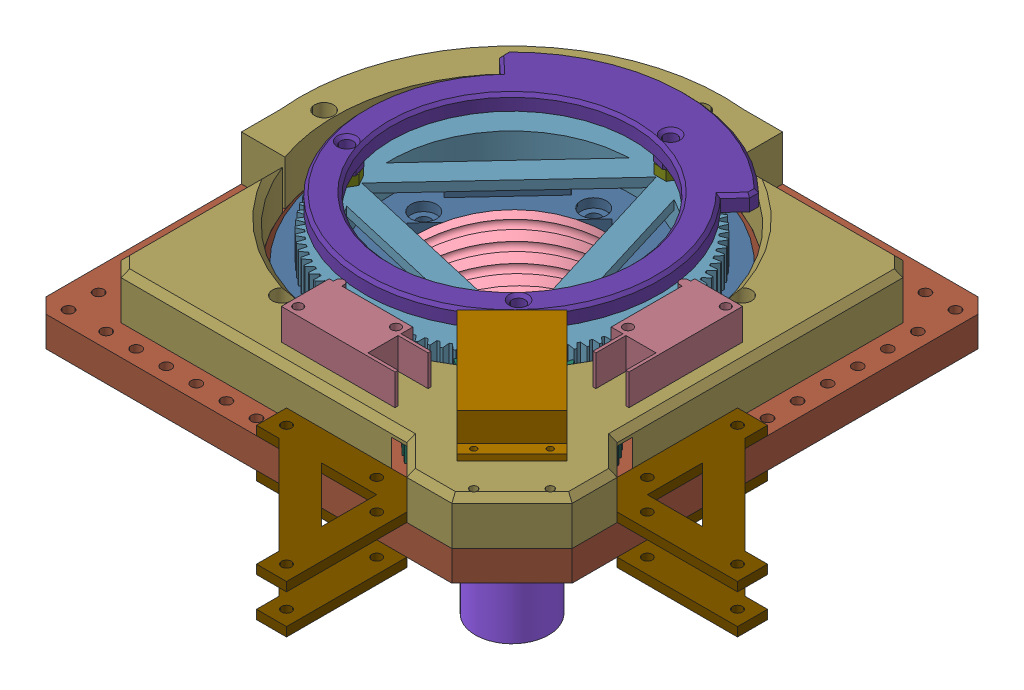
SolidWorks assembly st2, configuration ﾃﾞﾌｫﾙﾄ. Lengths in mm.
Overall size (210.56 112.16 211.97).
31 component instances, 21 part files, 85 mates.
Components (placement in the parent):
- Copy of Copy of 足回りモータ^st2-1: Copy of Copy of 足回りモータ^st2 [ﾃﾞﾌｫﾙﾄ] at (79.5108 -23 78.8626) x (0 1 0) z (-0.681736 0 0.731598) size (42 98.4 42) (virtual)
- Part5^st2-1: Part5^st2 [ﾃﾞﾌｫﾙﾄ] at (79.5108 -23 78.8626) x (0 -1 0) z (0.731598 0 0.681736) size (52 54 43) (virtual)
- Copy of Part1^st2-1: Copy of Part1^st2 [ﾃﾞﾌｫﾙﾄ] at (22.0794 -18.9784 99.4229) x (-0.664493 0.223485 0.713094) z (0.731598 0 0.681736) size (72 72 12) (virtual)
- Part7^st2-1: Part7^st2 [ﾃﾞﾌｫﾙﾄ] at (76.7838 -23 81.789) x (0 1 0) z (-0.681736 0 0.731598) size (80 47 80) (virtual)
- Part8^st2-1: Part8^st2 [ﾃﾞﾌｫﾙﾄ] at (99.9955 -23 97.9512) x (-0.225106 0.943913 0.24157) z (0.731598 0 0.681736) size (26 26 8) (virtual)
- Part9^st2-1: Part9^st2 [ﾃﾞﾌｫﾙﾄ] at (99.9955 -23 97.9512) x (0 -1 0) z (0.731598 0 0.681736) size (43 40 11) (virtual)
- Copy of Assem4^st2-1: Copy of Assem4^st2 [ﾃﾞﾌｫﾙﾄ] at (210.0035 137.7188 42.496) x (0.981351 0 0.192225) z (-0.192225 0 0.981351) (virtual)
- Copy of Copy of Copy of Copy (3) of Part3^st2-2: Copy of Copy of Copy of Copy (3) of Part3^st2 [ﾃﾞﾌｫﾙﾄ] at (53.8238 4 130.3704) x (-0.805716 0 0.592302) z (0 1 0) size (13 13 5) (virtual)
- Part30^st2-1: Part30^st2 [ﾃﾞﾌｫﾙﾄ] at (123.033 8 123.033) x (0.965926 0 0.258819) z (0 -1 0) size (24.4 24.4 60.8) (virtual)
- Part31^st2-1: Part31^st2 [ﾃﾞﾌｫﾙﾄ] at (207.1082 34.5248 112.8909) x (-0.707107 0 0.707107) z (0 1 0) size (25.8 49.4 11.5) (virtual)
- Part37^st2-4: Part37^st2 [ﾃﾞﾌｫﾙﾄ] at (79.5108 2 78.8626) x (0.731598 0 0.681736) z (0 1 0) size (114 114 10) (virtual)
- Copy of Copy of Copy of Copy (3) of Part3^st2-5: Copy of Copy of Copy of Copy (3) of Part3^st2 [ﾃﾞﾌｫﾙﾄ] at (130.3704 4 53.8238) x (-0.998139 0 0.060972) z (0 1 0) size (13 13 5) (virtual)
- Copy of Copy of Copy of Copy (3) of Part3^st2-6: Copy of Copy of Copy of Copy (3) of Part3^st2 [ﾃﾞﾌｫﾙﾄ] at (70 4 7.5) x (-0.272865 0 0.962052) z (0 1 0) size (13 13 5) (virtual)
- Part38^st2-1: Part38^st2 [ﾃﾞﾌｫﾙﾄ] at (53.8238 9 130.3704) x (-0.805716 0 0.592302) z (0 1 0) (virtual)
- Part41^st2-1: Part41^st2 [ﾃﾞﾌｫﾙﾄ] at (123.033 10 123.033) x (-0.965926 0 -0.258819) z (0 1 0) (virtual)
- Part42^st2-1: Part42^st2 [ﾃﾞﾌｫﾙﾄ] at (70 0 70) x (1 0 0) z (0 1 0) size (160 160 10) (virtual)
- Part43^st2-1: Part43^st2 [ﾃﾞﾌｫﾙﾄ] at (70 10 70) x (1 0 0) z (0 1 0) size (160.35 160.35 16.41) (virtual)
- Part44^st2-1: Part44^st2 [ﾃﾞﾌｫﾙﾄ] at (67.2 25 143.9) x (1 0 0) z (0 1 0) size (37.8 18.1 10.3) (virtual)
- Part44^st2-2: Part44^st2 [ﾃﾞﾌｫﾙﾄ] at (143.9 35.3 67.2) x (0 0 1) z (0 -1 0) size (37.8 18.1 10.3) (virtual)
- Copy of Copy of Copy of Copy (3) of Part3^st2-7: Copy of Copy of Copy of Copy (3) of Part3^st2 [ﾃﾞﾌｫﾙﾄ] at (7.5 4 70) x (-0.805716 0 0.592302) z (0 1 0) size (13 13 5) (virtual)
- Copy of Assem2^st2-2: Copy of Assem2^st2 [ﾃﾞﾌｫﾙﾄ] at (23.556 -1 157.424) x (-0.292715 0 -0.9562) z (0.9562 0 -0.292715) size (101.97 10 101.97) (virtual)
- Part45^st2-1: Part45^st2 [ﾃﾞﾌｫﾙﾄ] at origin (virtual)
- Copy of Assem1^st2-2: Copy of Assem1^st2 [ﾃﾞﾌｫﾙﾄ] at (36.0355 -1 -27.651) x (0.965926 0 0.258819) z (-0.258819 0 0.965926) size (52 10 52.13) (virtual)
- Part46^st2-2: Part46^st2 [ﾃﾞﾌｫﾙﾄ] at (102.1903 22 99.9964) x (1 0 0) z (0 1 0) size (8.08 7 3.2) (virtual)
- Part46^st2-3: Part46^st2 [ﾃﾞﾌｫﾙﾄ] at (27.9272 22 82.8795) x (1 0 0) z (0 1 0) size (8.08 7 3.2) (virtual)
- Part46^st2-4: Part46^st2 [ﾃﾞﾌｫﾙﾄ] at (79.8825 22 27.1242) x (1 0 0) z (0 1 0) size (8.08 7 3.2) (virtual)
- Part47^st2-4: Part47^st2 [ﾃﾞﾌｫﾙﾄ] at (70 27.7 70) x (-0.681736 0 0.731598) z (0 1 0) size (107 106.99 7.75) (virtual)
- Part48^st2-1: Part48^st2 [ﾃﾞﾌｫﾙﾄ] at (80.9379 10 49.2133) x (1 0 0) z (0 1 0) size (50 50 3) (virtual)
- Part48^st2-2: Part48^st2 [ﾃﾞﾌｫﾙﾄ] at (80.9379 -3 49.2133) x (1 0 0) z (0 1 0) size (50 50 3) (virtual)
- Part48^st2-3: Part48^st2 [ﾃﾞﾌｫﾙﾄ] at (194.0621 -3 225.7867) x (-1 0 0) z (0 1 0) size (50 50 3) (virtual)
- Part48^st2-4: Part48^st2 [ﾃﾞﾌｫﾙﾄ] at (194.0621 10 225.7867) x (-1 0 0) z (0 1 0) size (50 50 3) (virtual)
Mates (geometry in assembly coordinates):
- 相対固定5: in place: plane of ? through (-112.9944 -0.3949 73.4466) normal (0.707107 0 0.707107); plane of ? through (-19.7739 0 -19.7739) normal (0.707107 0 0.707107); moOrthogonalPlaneRef_w of ? through (-112.9944 -0.3949 73.4466) normal (0.707107 0 0.707107); plane of ? through (-19.7739 0 -19.7739) normal (0 1 0); plane of ? through (-112.9944 -0.3949 73.4466) normal (0.707107 0 0.707107); plane of ? through (-19.7739 0 -19.7739) normal (0.707107 0 -0.707107); plane of Copy of Copy of 足回りモータ^st2-1 through (79.5108 -23 78.8626) normal (0.731598 0 0.681736); unknown of Part5^st2-1
- 一致27: coincident aligned: plane of Copy of Copy of 足回りモータ^st2-1; plane of Part5^st2-1
- 一致28: coincident aligned: moOrthogonalPlaneRef_w of Copy of Copy of 足回りモータ^st2-1; plane of Part5^st2-1 through (79.5108 -23 78.8626) normal (0.681736 0 -0.731598)
- 一致29: coincident anti-aligned: moOrthogonalPlaneRef_w of Copy of Copy of 足回りモータ^st2-1; plane of Part5^st2-1 through (79.5108 -23 78.8626) normal (0 -1 0)
- 同心円16: concentric anti-aligned: cylinder of Part5^st2-1 through (50.2468 -23 51.5931) axis (0.731598 0 0.681736) radius 25; cylinder of Copy of Part1^st2-1 through (67.8052 -23 67.9548) axis (-0.731598 0 -0.681736) radius 25
- 相対固定7: in place: plane of ? through (-22.8566 -14.0328 -4.7881) normal (0 -1 0); plane of ? through (0 -14.0328 0) normal (0 -1 0); plane of ? through (-22.8566 -14.0328 -4.7881) normal (0 -1 0); plane of ? through (0 -14.0328 0) normal (0 0 -1); plane of ? through (-22.8566 -14.0328 -4.7881) normal (0 -1 0); plane of ? through (0 -14.0328 0) normal (-1 0 0); plane of Copy of Copy of 足回りモータ^st2-1 through (76.7838 -23 81.789) normal (-0.681736 0 0.731598); unknown of Part7^st2-1
- 一致34: coincident aligned: plane of Copy of Copy of 足回りモータ^st2-1; plane of Part7^st2-1
- 一致35: coincident aligned: moOrthogonalPlaneRef_w of Copy of Copy of 足回りモータ^st2-1; plane of Part7^st2-1 through (76.7838 -23 81.789) normal (-0.731598 0 -0.681736)
- 一致36: coincident anti-aligned: moOrthogonalPlaneRef_w of Copy of Copy of 足回りモータ^st2-1; plane of Part7^st2-1 through (76.7838 -23 81.789) normal (0 1 0)
- 一致37: coincident anti-aligned: plane of Copy of Part1^st2-1 through (67.8052 -23 67.9548) normal (0.731598 0 0.681736); plane of Part7^st2-1 through (65.0783 -23 70.8812) normal (-0.731598 0 -0.681736)
- 同心円19: concentric anti-aligned: cylinder of Copy of Copy of 足回りモータ^st2-1 through (99.4834 -23 97.474) axis (-0.731598 0 -0.681736) radius 5; cylinder of Part8^st2-1 through (94.1427 -23 92.4973) axis (0.731598 0 0.681736) radius 5
- 距離1: distance = 50 mm anti-aligned: plane of Part5^st2-1 through (57.5628 -23 58.4105) normal (0.731598 0 0.681736); plane of Part9^st2-1 through (94.1427 -23 92.4973) normal (-0.731598 0 -0.681736)
- 同心円21: concentric aligned: cylinder of Part8^st2-1 through (94.1427 -23 92.4973) axis (0.731598 0 0.681736) radius 13; cylinder of Part9^st2-1 through (94.1427 -23 92.4973) axis (0.731598 0 0.681736) radius 13.15
- 一致52: coincident anti-aligned: plane of Part8^st2-1 through (99.9955 -23 97.9512) normal (0.731598 0 0.681736); plane of Part9^st2-1 through (99.9955 -23 97.9512) normal (-0.731598 0 -0.681736)
- 平行1: parallel aligned: plane of Part5^st2-1 through (39.156 -23 78.1636) normal (-0.681736 0 0.731598); plane of Part9^st2-1 through (89.9191 2 113.1652) normal (-0.681736 0 0.731598)
- 相対固定17: in place: plane of ? through (-1.91 58.2582 -8.9277) normal (0 1 0); plane of ? through (0 58.2582 0) normal (0 1 0); plane of ? through (-1.91 58.2582 -8.9277) normal (0 1 0); plane of ? through (0 58.2582 0) normal (0 0 -1); plane of ? through (-1.91 58.2582 -8.9277) normal (0 1 0); plane of ? through (0 58.2582 0) normal (1 0 0); plane of Part5^st2-1 through (57.5628 2 58.4105) normal (0 1 0); unknown of Part37^st2-4
- 一致124: coincident aligned: plane of Part5^st2-1; plane of Part37^st2-4
- 一致125: coincident aligned: moOrthogonalPlaneRef_w of Part5^st2-1; plane of Part37^st2-4 through (79.5108 2 78.8626) normal (0.681736 0 -0.731598)
- 一致126: coincident anti-aligned: moOrthogonalPlaneRef_w of Part5^st2-1; plane of Part37^st2-4 through (79.5108 2 78.8626) normal (0.731598 0 0.681736)
- 相対固定18: in place: plane of ? through (3.002 101.7279 52.4706) normal (0 1 0); plane of ? through (0 101.7279 0) normal (0 1 0); plane of ? through (3.002 101.7279 52.4706) normal (0 1 0); plane of ? through (0 101.7279 0) normal (0 0 -1); plane of ? through (3.002 101.7279 52.4706) normal (0 1 0); plane of ? through (0 101.7279 0) normal (1 0 0); plane of Copy of Copy of Copy of Copy (3) of Part3^st2-2 through (53.8238 9 130.3704) normal (0 1 0); unknown of Part38^st2-1
- 一致135: coincident aligned: plane of Copy of Copy of Copy of Copy (3) of Part3^st2-2; plane of Part38^st2-1
- 一致136: coincident aligned: moOrthogonalPlaneRef_w of Copy of Copy of Copy of Copy (3) of Part3^st2-2; plane of Part38^st2-1 through (53.8238 9 130.3704) normal (0.592302 0 0.805716)
- 一致137: coincident anti-aligned: moOrthogonalPlaneRef_w of Copy of Copy of Copy of Copy (3) of Part3^st2-2; plane of Part38^st2-1 through (53.8238 9 130.3704) normal (-0.805716 0 0.592302)
- 一致169: coincident aligned: plane of Copy of Copy of Copy of Copy (3) of Part3^st2-2 through (53.8238 9 130.3704) normal (0 1 0); plane of Copy of Copy of Copy of Copy (3) of Part3^st2-5 through (130.3704 9 53.8238) normal (0 1 0)
- 一致170: coincident aligned: plane of Copy of Copy of Copy of Copy (3) of Part3^st2-5 through (130.3704 9 53.8238) normal (0 1 0); plane of Copy of Copy of Copy of Copy (3) of Part3^st2-6 through (70 9 7.5) normal (0 1 0)
- 一致175: coincident anti-aligned: plane of Part37^st2-4 through (70 9 70) normal (0 -1 0); plane of Copy of Copy of Copy of Copy (3) of Part3^st2-6 through (70 9 7.5) normal (0 1 0)
- 正接7: tangent anti-aligned: cylinder of Copy of Copy of Copy of Copy (3) of Part3^st2-2 through (53.8238 9 130.3704) axis (0 -1 0) radius 6.5; cylinder of Part37^st2-4 through (70 3.9 70) axis (0 1 0) radius 56
- 正接8: tangent anti-aligned: cylinder of Part37^st2-4 through (70 3.9 70) axis (0 1 0) radius 56; cylinder of Copy of Copy of Copy of Copy (3) of Part3^st2-5 through (130.3704 9 53.8238) axis (0 -1 0) radius 6.5
- 正接9: tangent anti-aligned: cylinder of Part37^st2-4 through (70 3.9 70) axis (0 1 0) radius 56; cylinder of Copy of Copy of Copy of Copy (3) of Part3^st2-6 through (70 9 7.5) axis (0 -1 0) radius 6.5
- 相対固定22: in place: plane of ? through (75.0873 50.8355 4.34) normal (-0.000638 0.999988 0.004853); plane of ? through (-0.0324 50.8075 0.2466) normal (-0.000638 0.999988 0.004853); plane of ? through (75.0873 50.8355 4.34) normal (-0.000638 0.999988 0.004853); plane of ? through (-0.0324 50.8075 0.2466) normal (0 0.004853 -0.999988); plane of ? through (75.0873 50.8355 4.34) normal (-0.000638 0.999988 0.004853); plane of ? through (-0.0324 50.8075 0.2466) normal (1 0.000638 0.000003); plane of Part30^st2-1 through (123.033 10 123.033) normal (0 1 0); unknown of Part41^st2-1
- 一致178: coincident aligned: plane of Part30^st2-1; plane of Part41^st2-1
- 一致179: coincident aligned: moOrthogonalPlaneRef_w of Part30^st2-1; plane of Part41^st2-1 through (123.033 10 123.033) normal (-0.258819 0 0.965926)
- 一致180: coincident anti-aligned: moOrthogonalPlaneRef_w of Part30^st2-1; plane of Part41^st2-1 through (123.033 10 123.033) normal (-0.965926 0 -0.258819)
- 一致184: coincident anti-aligned: plane of Part37^st2-4 through (70 2 70) normal (0 -1 0); plane of Part42^st2-1 through (70 2 70) normal (0 1 0)
- 同心円76: concentric aligned: cylinder of Part37^st2-4 through (70 12 70) axis (0 -1 0) radius 57; cylinder of Part42^st2-1 through (70 2 70) axis (0 -1 0) radius 70
- 同心円79: concentric aligned: cylinder of Copy of Copy of Copy of Copy (3) of Part3^st2-6 through (70 9 7.5) axis (0 -1 0) radius 3; cylinder of Part42^st2-1 through (70 2 7.5) axis (0 -1 0) radius 3.15
- 同心円80: concentric aligned: cylinder of Copy of Copy of Copy of Copy (3) of Part3^st2-2 through (53.8238 9 130.3704) axis (0 -1 0) radius 3; cylinder of Part42^st2-1 through (53.8238 2 130.3704) axis (0 -1 0) radius 3.15
- 同心円81: concentric aligned: cylinder of Copy of Copy of Copy of Copy (3) of Part3^st2-5 through (130.3704 9 53.8238) axis (0 -1 0) radius 3; cylinder of Part42^st2-1 through (130.3704 2 53.8238) axis (0 -1 0) radius 3.15
- 同心円82: concentric anti-aligned: cylinder of Part30^st2-1 through (123.033 -35.8 123.033) axis (0 1 0) radius 12.2; cylinder of Part42^st2-1 through (123.033 2 123.033) axis (0 -1 0) radius 12.25
- 同心円83: concentric aligned: cylinder of Part30^st2-1 through (116.3155 3 116.3155) axis (0 1 0) radius 1.5; cylinder of Part42^st2-1 through (116.3155 8 116.3155) axis (0 1 0) radius 1.7
- 相対固定24: in place: plane of ? through (-0.444 58.3221 58.4194) normal (-0.000638 0.999988 0.004853); plane of ? through (-0.0374 58.6044 0.2844) normal (-0.000638 0.999988 0.004853); plane of ? through (-0.444 58.3221 58.4194) normal (-0.000638 0.999988 0.004853); plane of ? through (-0.0374 58.6044 0.2844) normal (0 0.004853 -0.999988); plane of ? through (-0.444 58.3221 58.4194) normal (-0.000638 0.999988 0.004853); plane of ? through (-0.0374 58.6044 0.2844) normal (1 0.000638 0.000003); plane of Part42^st2-1 through (70 10 70) normal (0 1 0); unknown of Part43^st2-1
- 一致185: coincident aligned: plane of Part42^st2-1; plane of Part43^st2-1
- 一致186: coincident aligned: moOrthogonalPlaneRef_w of Part42^st2-1; plane of Part43^st2-1 through (70 10 70) normal (0 0 -1)
- 一致187: coincident anti-aligned: moOrthogonalPlaneRef_w of Part42^st2-1; plane of Part43^st2-1 through (70 10 70) normal (1 0 0)
- 一致192: coincident anti-aligned: plane of Part43^st2-1 through (70 25 70) normal (0 1 0); plane of Part44^st2-1 through (67.2 25 143.9) normal (0 -1 0)
- 同心円85: concentric anti-aligned: cylinder of Part43^st2-1 through (70 10 141.1) axis (0 1 0) radius 1.7; cylinder of Part44^st2-1 through (70 35.3 141.1) axis (0 -1 0) radius 1.55
- 同心円86: concentric anti-aligned: cylinder of Part43^st2-1 through (92.2 10 130.8) axis (0 1 0) radius 1.7; cylinder of Part44^st2-1 through (92.2 35.3 130.8) axis (0 -1 0) radius 1.55
- 一致193: coincident anti-aligned: plane of Part42^st2-1 through (70 2 0) normal (0 0 -1)
- 一致194: coincident anti-aligned: plane of Part42^st2-1 through (0 2 70) normal (-1 0 0)
- 一致196: coincident anti-aligned: plane of Part42^st2-1 through (70 0 70) normal (0 -1 0)
- 同心円87: concentric aligned: cylinder of Part31^st2-1 through (141.4178 34.5238 154.1457) axis (0 1 0) radius 1; cylinder of Part43^st2-1 through (141.4178 10 154.1457) axis (0 1 0) radius 1.25
- 同心円89: concentric aligned: cylinder of Part31^st2-1 through (154.1457 34.5238 141.4178) axis (0 1 0) radius 1; cylinder of Part43^st2-1 through (154.1457 10 141.4178) axis (0 1 0) radius 1.25
- 同心円90: concentric aligned: cylinder of Part43^st2-1 through (141.1 10 70) axis (0 1 0) radius 1.7; cylinder of Part44^st2-2 through (141.1 25 70) axis (0 1 0) radius 1.55
- 同心円91: concentric aligned: cylinder of Part43^st2-1 through (130.8 10 92.2) axis (0 1 0) radius 1.7; cylinder of Part44^st2-2 through (130.8 25 92.2) axis (0 1 0) radius 1.55
- 一致198: coincident anti-aligned: plane of Part43^st2-1 through (70 25 70) normal (0 1 0); plane of Part44^st2-2 through (143.9 25 67.2) normal (0 -1 0)
- 一致200: coincident anti-aligned: plane of Part42^st2-1 through (70 4 70) normal (0 1 0); plane of Copy of Copy of Copy of Copy (3) of Part3^st2-7 through (7.5 4 70) normal (0 -1 0)
- 一致201: coincident anti-aligned: plane of Part42^st2-1 through (70 4 70) normal (0 1 0); plane of Copy of Copy of Copy of Copy (3) of Part3^st2-7 through (7.5 4 70) normal (0 -1 0)
- 同心円94: concentric aligned: cylinder of Part42^st2-1 through (7.5 2 70) axis (0 -1 0) radius 3.15; cylinder of Copy of Copy of Copy of Copy (3) of Part3^st2-7 through (7.5 9 70) axis (0 -1 0) radius 3
- 同心円97: concentric aligned: cylinder of Part37^st2-4 through (102.1903 2 99.9964) axis (0 1 0) radius 2.15; cylinder of Copy of Assem2^st2-2 through (102.1903 12 99.9964) axis (0 1 0) radius 2.15
- 同心円98: concentric aligned: cylinder of Part37^st2-4 through (79.8825 2 27.1242) axis (0 1 0) radius 2.15; cylinder of Copy of Assem2^st2-2 through (79.8825 12 27.1242) axis (0 1 0) radius 2.15
- 一致203: coincident anti-aligned: plane of Part37^st2-4 through (70 12 70) normal (0 1 0); plane of Copy of Assem2^st2-2 through (70 12 70) normal (0 -1 0)
- 同心円103: concentric aligned: cylinder of Part30^st2-1 through (119.8752 16 134.8183) axis (0.258819 0 -0.965926) radius 1.5; cylinder of Copy of Assem1^st2-2 through (116.3067 16 148.1358) axis (0.258819 0 -0.965926) radius 1.65
- 同心円106: concentric anti-aligned: cylinder of Part30^st2-1 through (123.033 25 123.033) axis (0 -1 0) radius 3; cylinder of Copy of Assem1^st2-2 through (123.033 -28.0001 123.033) axis (0 1 0) radius 3
- 一致214: coincident anti-aligned: plane of Part30^st2-1 through (123.033 8 123.033) normal (0 1 0); plane of Part42^st2-1 through (70 8 70) normal (0 -1 0)
- 一致218: coincident anti-aligned: plane of Copy of Assem2^st2-2 through (70 22 70) normal (0 1 0); plane of Part46^st2-2 through (102.1903 22 99.9964) normal (0 -1 0)
- 同心円108: concentric anti-aligned: cylinder of Copy of Assem2^st2-2 through (102.1903 12 99.9964) axis (0 1 0) radius 2.15; cylinder of Part46^st2-2 through (102.1903 25.2 99.9964) axis (0 -1 0) radius 2
- 一致219: coincident anti-aligned: plane of Copy of Assem2^st2-2 through (70 22 70) normal (0 1 0); plane of Part46^st2-3 through (27.9272 22 82.8795) normal (0 -1 0)
- 一致220: coincident anti-aligned: plane of Copy of Assem2^st2-2 through (70 22 70) normal (0 1 0); plane of Part46^st2-4 through (79.8825 22 27.1242) normal (0 -1 0)
- 同心円109: concentric anti-aligned: cylinder of Copy of Assem2^st2-2 through (79.8825 12 27.1242) axis (0 1 0) radius 2.15; cylinder of Part46^st2-4 through (79.8825 25.2 27.1242) axis (0 -1 0) radius 2
- 同心円110: concentric anti-aligned: cylinder of Copy of Assem2^st2-2 through (27.9272 12 82.8795) axis (0 1 0) radius 2.15; cylinder of Part46^st2-3 through (27.9272 25.2 82.8795) axis (0 -1 0) radius 2
- 同心円113: concentric anti-aligned: cylinder of Copy of Assem2^st2-2 through (70 -28.0001 70) axis (0 1 0) radius 40; cylinder of Part47^st2-4 through (70 32.7 70) axis (0 -1 0) radius 40
- 同心円114: concentric anti-aligned: cylinder of Copy of Assem2^st2-2 through (102.1903 12 99.9964) axis (0 1 0) radius 2.15; cylinder of Part47^st2-4 through (102.1903 32.7 99.9964) axis (0 -1 0) radius 2.15
- 同心円115: concentric anti-aligned: cylinder of Part42^st2-1 through (110 -0.001 155) axis (0 1 0) radius 1.75; cylinder of Part48^st2-1 through (110 13 155) axis (0 -1 0) radius 1.65
- 一致229: coincident anti-aligned: plane of Part42^st2-1 through (70 10 70) normal (0 1 0); plane of Part48^st2-1 through (80.9379 10 49.2133) normal (0 -1 0)
- 同心円116: concentric anti-aligned: cylinder of Part42^st2-1 through (80 -0.001 155) axis (0 1 0) radius 1.75; cylinder of Part48^st2-1 through (80 13 155) axis (0 -1 0) radius 1.65
- 同心円117: concentric anti-aligned: cylinder of Part42^st2-1 through (110 -0.001 155) axis (0 1 0) radius 1.75; cylinder of Part48^st2-2 through (110 0 155) axis (0 -1 0) radius 1.65
- 一致230: coincident anti-aligned: plane of Part42^st2-1 through (70 0 70) normal (0 -1 0); plane of Part48^st2-2 through (80.9379 0 49.2133) normal (0 1 0)
- 同心円118: concentric anti-aligned: cylinder of Part42^st2-1 through (80 -0.001 155) axis (0 1 0) radius 1.75; cylinder of Part48^st2-2 through (80 0 155) axis (0 -1 0) radius 1.65
- 同心円119: concentric aligned: cylinder of Part48^st2-3 through (155 0 110) axis (0 -1 0) radius 1.65; cylinder of Part48^st2-4 through (155 13 110) axis (0 -1 0) radius 1.65
- 同心円120: concentric anti-aligned: cylinder of Part42^st2-1 through (155 -0.001 110) axis (0 1 0) radius 1.75; cylinder of Part48^st2-3 through (155 0 110) axis (0 -1 0) radius 1.65
- 同心円121: concentric aligned: cylinder of Part48^st2-3 through (155 0 80) axis (0 -1 0) radius 1.65; cylinder of Part48^st2-4 through (155 13 80) axis (0 -1 0) radius 1.65
- 同心円122: concentric anti-aligned: cylinder of Part42^st2-1 through (155 -0.001 80) axis (0 1 0) radius 1.75; cylinder of Part48^st2-4 through (155 13 80) axis (0 -1 0) radius 1.65
- 一致231: coincident anti-aligned: plane of Part42^st2-1 through (70 10 70) normal (0 1 0); plane of Part48^st2-4 through (194.0621 10 225.7867) normal (0 -1 0)
- 一致232: coincident anti-aligned: plane of Part42^st2-1 through (70 0 70) normal (0 -1 0); plane of Part48^st2-3 through (194.0621 0 225.7867) normal (0 1 0)
- 一致233: coincident anti-aligned: plane of Part46^st2-2 through (102.1903 25.2 99.9964) normal (0 1 0); plane of Part47^st2-4 through (70 25.2 70) normal (0 -1 0)
